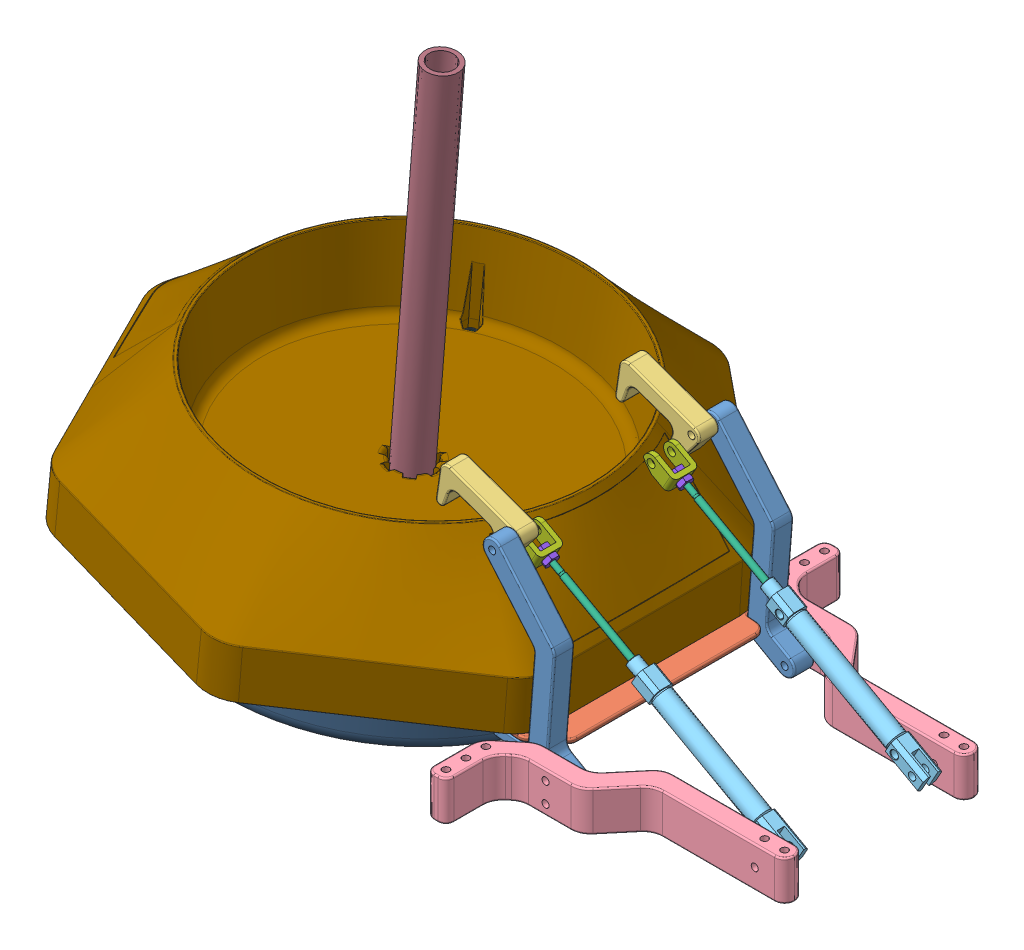
SolidWorks assembly Mogo_Intake_Assembly, configuration Default. Lengths in mm.
Overall size (471.42 326.71 329.62).
40 component instances, 16 part files, 25 mates.
Components (placement in the parent):
- Mogo_Intake_Pivot_Arm-1: Mogo_Intake_Pivot_Arm [Default] at (-42.0151 50.5778 119.045) x (0 0 1) z (-0.996797 0.079974 0) size (12.7 119 68.1)
- Mogo_Intake_Pivot_Arm-2: Mogo_Intake_Pivot_Arm [Default] at (-42.0151 50.5778 -20.655) x (0 0 1) z (-0.996797 0.079974 0) size (12.7 119 68.1)
- Mogo_Adapt_Flat-1: Mogo_Adapt_Flat [Default] at (-218.2422 76.0531 55.545) x (0 0 -1) z (0.996797 -0.079974 0) size (152.4 3 57.83)
- Mogo_Intake_Hook-1: Mogo_Intake_Hook [Default] at (-88.7364 160.9679 119.045) x (0 0 -1) z (0.942133 -0.335239 0) size (12.7 25 53.9)
- Mogo_Intake_Hook-2: Mogo_Intake_Hook [Default] at (-88.7364 160.9679 4.745) x (0 0 -1) z (0.942133 -0.335239 0) size (12.7 25 53.9)
- Chassis_Mount-1: Chassis_Mount [Default] at (-73.7651 44.2278 176.195) size (165.1 25.4 76.2)
- Chassis_Mount-2: Chassis_Mount [Default] at (-73.7651 69.6278 -65.105) x (1 0 0) z (0 0 -1) size (165.1 25.4 76.2)
- PistonWithHead-1: PistonWithHead [Default] at (57.9083 120.3309 109.8748) x (0.486638 0.873604 0) z (-0.873604 0.486638 0) size (13.68 16 199.2) (flexible)
  - PistonAssembly-1: PistonAssembly [Default] at (3.7639 -3.8574 -3.1657) size (13.68 13.68 185.84) (flexible)
    - Bi-directional Cylinder Main v1-1: Bi-directional Cylinder Main v1 [Default] at (-55.247 15.3872 20.1993) size (12 12 118.8)
    - Bi-directional Cylinder Shaft v1-1: Bi-directional Cylinder Shaft v1 [Default] at (-55.247 15.3872 67.2429) x (-0.862683 -0.505745 0) z (0 0 1) size (10 10 105.8)
  - PistonHeadBracket-1: PistonHeadBracket [Default] at (-46.4831 19.5298 155.3316) x (0 -1 0) z (-1 0 0) size (16 19.15 10)
  - Bi-directional Cylinder Nut v1-1: Bi-directional Cylinder Nut v1 [Default] at (-51.4831 11.5298 70.1802) x (-0.5 -0.866025 0) z (0 0 1) size (8.86 9.11 2.81)
  - Bi-directional Cylinder Nut v1-2: Bi-directional Cylinder Nut v1 [Default] at (-51.4831 11.5298 64.3862) x (0.5 -0.866025 0) z (0 0 1) size (8.86 9.11 2.81)
- PistonWithHead-2: PistonWithHead [Default] at (7.801 30.3792 1.2152) x (-0.486638 -0.873604 0) z (-0.873604 0.486638 0) size (13.68 16 199.2) (flexible)
  - PistonAssembly-1: PistonAssembly [Default] at (3.7639 -3.8574 -3.1657) size (13.68 13.68 185.84) (flexible)
    - Bi-directional Cylinder Main v1-1: Bi-directional Cylinder Main v1 [Default] at (-55.247 15.3872 20.1993) size (12 12 118.8)
    - Bi-directional Cylinder Shaft v1-1: Bi-directional Cylinder Shaft v1 [Default] at (-55.247 15.3872 67.2429) x (-0.862683 -0.505745 0) z (0 0 1) size (10 10 105.8)
  - PistonHeadBracket-1: PistonHeadBracket [Default] at (-46.4831 19.5298 155.3316) x (0 -1 0) z (-1 0 0) size (16 19.15 10)
  - Bi-directional Cylinder Nut v1-1: Bi-directional Cylinder Nut v1 [Default] at (-51.4831 11.5298 70.1802) x (-0.5 -0.866025 0) z (0 0 1) size (8.86 9.11 2.81)
  - Bi-directional Cylinder Nut v1-2: Bi-directional Cylinder Nut v1 [Default] at (-51.4831 11.5298 64.3862) x (0.5 -0.866025 0) z (0 0 1) size (8.86 9.11 2.81)
- BlueMogo-1: BlueMogo [Default] at (-217.4944 85.3731 55.545) x (0.996797 -0.079974 0) z (0 0 1) size (329.62 312.25 329.62)
  - BlueMogo.step-1: BlueMogo.step [Default] at origin size (329.62 312.25 329.62)
    - 276-7048-270 Rev3_Red.step-1: 276-7048-270 Rev3_Red.step [Default] x (0 0 -1) z (1 0 0) size (329.62 312.25 329.62)
      - 276-7048-203 Rev5_Yellow.step-1: 276-7048-203 Rev5_Yellow.step [Default] at origin size (322.53 130.15 315.74)
      - 276-7048-204 Rev5.step-1: 276-7048-204 Rev5.step [Default] at (0 -0.25 0) x (-1 0 0) z (0 0 -1) size (260.2 58 260.2)
      - 276-7048-205 Rev1.step-1: 276-7048-205 Rev1.step [Default] at (0 -18.506 0) x (-0.5 0 0.866025) z (0 -1 0) size (241.3 241.3 2)
      - 276-6089-013 Rev4.step-1: 276-6089-013 Rev4.step [Default] at (0 -46.7356 0) x (-0.981976 0 -0.189007) z (0.189007 0 -0.981976) size (60.39 14.6 24.66)
      - 276-6089-013 Rev4.step-2: 276-6089-013 Rev4.step [Default] at (0 -46.7356 0) x (0.981976 0 0.189007) z (-0.189007 0 0.981976) size (60.39 14.6 24.66)
      - 276-7048-209 Rev2.step-1: 276-7048-209 Rev2.step [Default] at (0 101.6 0) x (0.577811 0 0.816171) z (0 1 0) size (21.3 21.3 304.8)
      - 276-1027-001.step-1: 276-1027-001.step [Default] at (-87.9864 15.4 -50.799) x (0.866025 0 -0.5) z (0.5 0 0.866025) size (8.61 5.64 9.94)
      - 276-4999-001 Rev1_No Threads.step-1: 276-4999-001 Rev1_No Threads.step [Default] at (-87.9882 -23.046 -50.8) x (-0.837169 0 -0.546944) z (-0.546944 0 0.837169) size (7.92 46.66 7.92)
      - 276-4993-001 Rev1_No Threads.step-1: 276-4993-001 Rev1_No Threads.step [Default] at (21.0263 -46.7356 8.3751) x (0.527907 -0.843202 0.10161) z (-0.828004 -0.537597 -0.159371) size (7.92 18.09 7.92)
      - 276-1027-001.step-2: 276-1027-001.step [Default] at (87.9864 15.4 -50.799) x (0 0 1) z (-1 0 0) size (8.61 5.64 9.94)
      - 276-1027-001.step-3: 276-1027-001.step [Default] at (0 15.4 101.5979) x (0.866025 0 0.5) z (-0.5 0 0.866025) size (8.61 5.64 9.94)
      - 276-1027-001.step-4: 276-1027-001.step [Default] at (-22.6328 -46.7356 -0.0283) x (0 1 0) z (0.981976 0 0.189007) size (8.61 5.64 9.94)
      - 276-1027-001.step-5: 276-1027-001.step [Default] at (22.6328 -46.7356 0.0283) x (0 1 0) z (-0.981976 0 -0.189007) size (8.61 5.64 9.94)
      - 276-4993-001 Rev1_No Threads.step-2: 276-4993-001 Rev1_No Threads.step [Default] at (-21.0263 -46.7356 -8.3751) x (-0.837157 0.52269 -0.161133) z (-0.513268 -0.852523 -0.098792) size (7.92 18.09 7.92)
      - 276-4999-001 Rev1_No Threads.step-2: 276-4999-001 Rev1_No Threads.step [Default] at (87.9882 -23.046 -50.8) x (-0.925243 0 -0.379375) z (-0.379375 0 0.925243) size (7.92 46.66 7.92)
      - 276-4999-001 Rev1_No Threads.step-3: 276-4999-001 Rev1_No Threads.step [Default] at (0 -23.046 101.6) x (-0.985271 0 -0.170998) z (-0.170998 0 0.985271) size (7.92 46.66 7.92)
Mates (geometry in assembly coordinates):
- Concentric1: concentric anti-aligned: circle of Mogo_Intake_Pivot_Arm-1; circle of Mogo_Adapt_Flat-1
- Concentric2: concentric anti-aligned: circle of Mogo_Intake_Pivot_Arm-1; circle of Mogo_Adapt_Flat-1
- Concentric3: concentric anti-aligned: circle of Mogo_Intake_Pivot_Arm-2; circle of Mogo_Adapt_Flat-1
- Concentric4: concentric anti-aligned: circle of Mogo_Intake_Pivot_Arm-2; circle of Mogo_Adapt_Flat-1
- Coincident4: coincident anti-aligned: plane of Mogo_Intake_Pivot_Arm-2 through (-41.1114 61.8416 -7.955) normal (0.079974 0.996797 0); plane of Mogo_Adapt_Flat-1 through (-218.2422 76.0531 55.545) normal (-0.079974 -0.996797 0)
- Coincident6: coincident anti-aligned: plane of Mogo_Intake_Pivot_Arm-1 through (-41.1114 61.8416 131.745) normal (0.079974 0.996797 0); plane of Mogo_Adapt_Flat-1 through (-218.2422 76.0531 55.545) normal (-0.079974 -0.996797 0)
- Coincident11: coincident anti-aligned: plane of Mogo_Intake_Pivot_Arm-1 through (-42.0151 50.5778 119.045) normal (0 0 -1); plane of Mogo_Intake_Hook-1 through (-88.7364 160.9679 119.045) normal (0 0 1)
- Coincident12: coincident anti-aligned: plane of Mogo_Intake_Pivot_Arm-2 through (-42.0151 50.5778 -7.955) normal (0 0 1); plane of Mogo_Intake_Hook-2 through (-88.7364 160.9679 -7.955) normal (0 0 -1)
- Coincident13: coincident aligned: plane of Mogo_Intake_Hook-1 through (-87.0602 165.6786 106.345) normal (0.335239 0.942133 0); plane of Mogo_Intake_Hook-2 through (-87.0602 165.6786 -7.955) normal (0.335239 0.942133 0)
- Concentric6: concentric aligned: cylinder of Mogo_Intake_Pivot_Arm-1 through (-42.0151 50.5778 131.745) axis (0 0 -1) radius 2.25; cylinder of Chassis_Mount-1 through (-42.0151 50.5778 182.545) axis (0 0 -1) radius 2.25
- Coincident18: coincident aligned: plane of Chassis_Mount-1 through (-73.7651 69.6278 176.195) normal (0 1 0); plane of Chassis_Mount-2 through (-73.7651 69.6278 -65.105) normal (0 1 0)
- Concentric7: concentric anti-aligned: cylinder of Chassis_Mount-1 through (-42.0151 50.5778 182.545) axis (0 0 -1) radius 2.25; cylinder of Chassis_Mount-2 through (-42.0151 50.5778 -71.455) axis (0 0 1) radius 2.25
- Distance1: distance = 241.3 mm: cylinder of Chassis_Mount-1 through (-73.7651 69.6278 176.195) axis (0 -1 0) radius 2.25; cylinder of Chassis_Mount-2 through (-73.7651 44.2278 -65.105) axis (0 1 0) radius 2.25
- Concentric9: concentric anti-aligned: cylinder of Chassis_Mount-2 through (65.9349 56.9278 -71.455) axis (0 0 1) radius 2.25; cylinder of PistonWithHead-2/PistonAssembly-1/Bi-directional Cylinder Main v1-1 through (65.9349 56.9278 12.745) axis (0 0 -1) radius 2.39
- Concentric11: concentric aligned: cylinder of Mogo_Intake_Hook-2 through (-98.4756 148.5121 -7.955) axis (0 0 1) radius 2.25; cylinder of PistonWithHead-2/PistonHeadBracket-1 through (-98.4756 148.5121 4.745) axis (0 0 1) radius 2.5
- Concentric12: concentric anti-aligned: cylinder of Chassis_Mount-1 through (65.9349 56.9278 182.545) axis (0 0 -1) radius 2.25; cylinder of PistonWithHead-1/PistonAssembly-1/Bi-directional Cylinder Main v1-1 through (65.9349 56.9278 98.345) axis (0 0 1) radius 2.39
- Concentric13: concentric anti-aligned: cylinder of Mogo_Intake_Hook-1 through (-98.4756 148.5121 106.345) axis (0 0 1) radius 2.25; cylinder of PistonWithHead-1/PistonHeadBracket-1 through (-98.4756 148.5121 106.345) axis (0 0 -1) radius 2.5
- Coincident20: coincident anti-aligned: plane of Mogo_Intake_Hook-1 through (-88.7364 160.9679 106.345) normal (0 0 -1); plane of PistonWithHead-1/PistonHeadBracket-1 through (-105.2768 146.5773 106.345) normal (0 0 1)
- Coincident21: coincident anti-aligned: plane of Mogo_Intake_Hook-2 through (-88.7364 160.9679 4.745) normal (0 0 1); plane of PistonWithHead-2/PistonHeadBracket-1 through (-100.4105 155.3133 4.745) normal (0 0 -1)
- Coincident22: coincident anti-aligned: plane of Mogo_Intake_Pivot_Arm-2 through (-42.0151 50.5778 -20.655) normal (0 0 -1); plane of Chassis_Mount-2 through (-73.7651 44.2278 -20.655) normal (0 0 1)
- Concentric14: concentric aligned: cylinder of Mogo_Intake_Pivot_Arm-1 through (-88.7364 160.9679 131.745) axis (0 0 -1) radius 2.25; circle of Mogo_Intake_Hook-1
- Concentric15: concentric aligned: cylinder of Mogo_Intake_Pivot_Arm-2 through (-88.7364 160.9679 -7.955) axis (0 0 -1) radius 2.25; circle of Mogo_Intake_Hook-2
- LimitAngle1: limit planar angle = 0.261799 rad aligned: plane of Mogo_Intake_Hook-1 through (-87.0602 165.6786 106.345) normal (0.335239 0.942133 0); plane of Mogo_Adapt_Flat-1 through (-218.0023 79.0435 55.545) normal (0.079974 0.996797 0)
- Concentric16: concentric anti-aligned: circle of Mogo_Adapt_Flat-1; cylinder of BlueMogo-1/BlueMogo.step-1/276-7048-270 Rev3_Red.step-1/276-7048-204 Rev5.step-1 through (-221.913 30.3001 55.545) axis (-0.079974 -0.996797 0) radius 127
- Coincident26: coincident anti-aligned: plane of Mogo_Adapt_Flat-1 through (-218.0023 79.0435 55.545) normal (0.079974 0.996797 0); plane of BlueMogo-1/BlueMogo.step-1/276-7048-270 Rev3_Red.step-1/276-7048-203 Rev5_Yellow.step-1 through (-93.323 69.0403 115.7803) normal (-0.079974 -0.996797 0)
